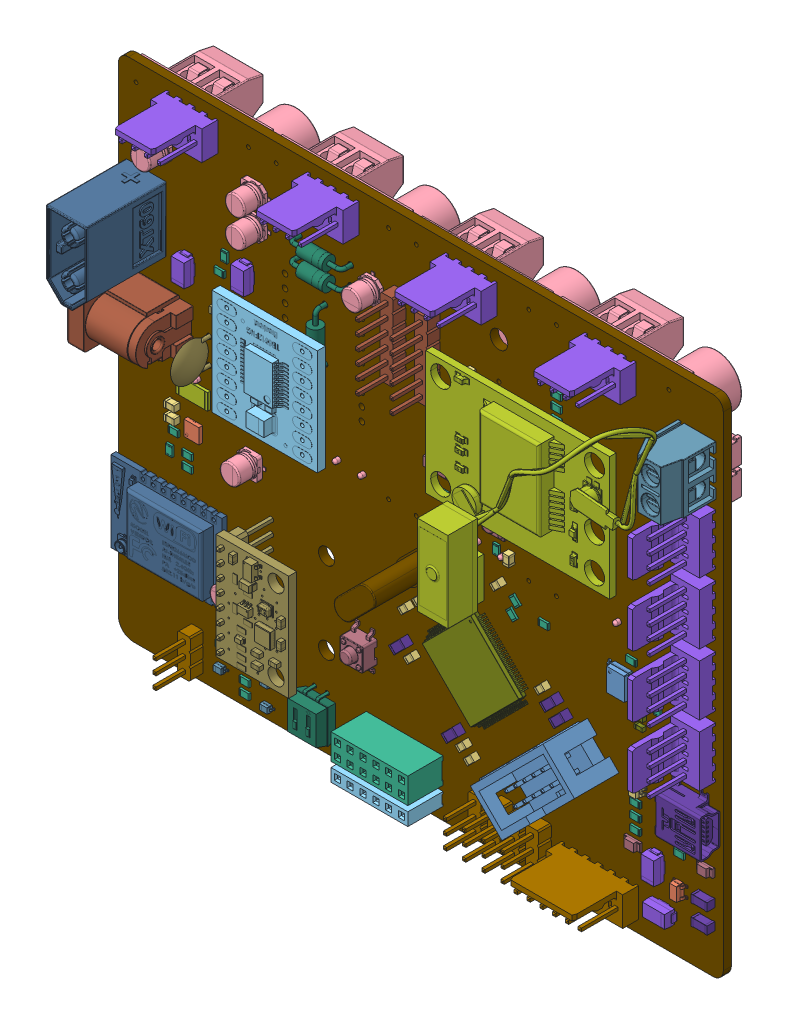
SolidWorks assembly noah_v02, configuration Default. Lengths in mm.
Overall size (125.96 104.91 49.76).
240 component instances, 36 part files, 0 mates.
Components (placement in the parent):
- noah_v02.step-1: noah_v02.step [Default] at origin size (125.96 104.91 49.76)
  - IDC-Header_2x05_P2.54mm_Vertical.step-1: IDC-Header_2x05_P2.54mm_Vertical.step [Default] at (176.6 -132.6 1.65) x (-0.707107 0.707107 0) z (0 0 1) size (9.1 20.36 12.1)
    - SOLID.step-1: SOLID.step [Default] at origin size (9.1 20.36 12.1)
  - DFN-8-1EP_3x3mm_P0.5mm_EP1.66x2.38mm.step-1: DFN-8-1EP_3x3mm_P0.5mm_EP1.66x2.38mm.step [Default] at (105.305 -107.385 1.65) x (0 1 0) z (0 0 1) size (3 2.98 0.77)
    - SOLID-0.step-1: SOLID-0.step [Default] at origin size (3 2.98 0.77)
  - C_0805_2012Metric.step-1: C_0805_2012Metric.step [Default] at (160.4 -70.1 1.65) x (0 -1 0) z (0 0 1) size (2 1.25 1.25)
    - SOLID-1.step-1: SOLID-1.step [Default] at origin size (2 1.25 1.25)
  - CP_Elec_4x4.5.step-1: CP_Elec_4x4.5.step [Default] at (140.6 -65.3 1.65) x (0 -1 0) z (0 0 1) size (5.74 5.46 4.5)
    - SOLID-2.step-1: SOLID-2.step [Default] at origin size (5.74 5.46 4.5)
  - C_0805_2012Metric.step-2: C_0805_2012Metric.step [Default] at (115.6 -134.6 1.65) size (2 1.25 1.25)
    - SOLID-1.step-1: SOLID-1.step [Default] at origin size (2 1.25 1.25)
  - CP_Elec_4x4.5.step-2: CP_Elec_4x4.5.step [Default] at (114.6 -129.4 1.65) x (0 1 0) z (0 0 1) size (5.74 5.46 4.5)
    - SOLID-2.step-1: SOLID-2.step [Default] at origin size (5.74 5.46 4.5)
  - PinSocket_1x06_P2.54mm_Vertical.step-1: PinSocket_1x06_P2.54mm_Vertical.step [Default] at (153.2 -146.2 1.65) x (0 -1 0) z (0 0 1) size (2.54 15.24 10.1)
    - SOLID-3.step-1: SOLID-3.step [Default] at origin size (2.54 15.24 10.1)
  - PinSocket_2x06_P2.54mm_Vertical.step-1: PinSocket_2x06_P2.54mm_Vertical.step [Default] at (153.2 -142.6 1.65) x (0 -1 0) z (0 0 1) size (5.08 15.24 10.1)
    - SOLID-4.step-1: SOLID-4.step [Default] at origin size (5.08 15.24 10.1)
  - ublox_NEO-6M.step-1: ublox_NEO-6M.step [Default] at (181.8 -59.6 11.65) x (0 1 0) z (1 0 0) size (39.06 22.61 48.01)
    - COMPOUND.step-1: COMPOUND.step [Default] at origin size (39.06 22.61 48.01)
  - D_SMA.step-1: D_SMA.step [Default] at (198.4 -143.2 1.65) x (-1 0 0) z (0 0 1) size (5 2.7 2.22)
    - SOLID-5.step-1: SOLID-5.step [Default] at origin size (5 2.7 2.22)
  - PinHeader_1x03_P2.54mm_Vertical.step-1: PinHeader_1x03_P2.54mm_Vertical.step [Default] at (105.6 -147.4 1.65) x (-1 0 0) z (0 0 1) size (2.54 7.62 11.54)
    - SOLID-6.step-1: SOLID-6.step [Default] at origin size (2.54 7.62 11.54)
  - C_0805_2012Metric.step-3: C_0805_2012Metric.step [Default] at (101.3 -107.1 1.65) x (-1 0 0) z (0 0 1) size (2 1.25 1.25)
    - SOLID-1.step-1: SOLID-1.step [Default] at origin size (2 1.25 1.25)
  - C_0805_2012Metric.step-4: C_0805_2012Metric.step [Default] at (101.3 -104.8 1.65) x (-1 0 0) z (0 0 1) size (2 1.25 1.25)
    - SOLID-1.step-1: SOLID-1.step [Default] at origin size (2 1.25 1.25)
  - ESP07.step-1: ESP07.step [Default] at (101.6 -127.3 1.65) x (0 1 0) z (1 0 0) size (19.34 14.61 27.24)
    - COMPOUND-7.step-1: COMPOUND-7.step [Default] at origin size (19.34 14.61 27.24)
  - Power_Barrel_Connector_Jack_694106301002.step-1: Power_Barrel_Connector_Jack_694106301002.step [Default] at (104.13 -90.01 1.65) x (0 -1 0) z (0 0 1) size (9.49 14.48 14.52)
    - COMPOUND-8.step-1: COMPOUND-8.step [Default] at origin size (9.49 14.48 14.52)
  - GY-91.step-1: GY-91.step [Default] at (119 -134.7 9.65) size (14.4 21 11.75)
    - COMPOUND-9.step-1: COMPOUND-9.step [Default] at origin size (14.4 21 11.75)
  - Tact_Switch_4.5mm_SMT.step-1: Tact_Switch_4.5mm_SMT.step [Default] at (139.14 -127.61 1.65) x (0 1 0) z (0 0 1) size (7.5 4.5 4.2)
    - COMPOUND-10.step-1: COMPOUND-10.step [Default] at origin size (7.5 4.5 4.2)
  - Tact_Switch_4.5mm_SMT.step-2: Tact_Switch_4.5mm_SMT.step [Default] at (167.3 -90.93 1.65) x (0 -1 0) z (0 0 1) size (7.5 4.5 4.2)
    - COMPOUND-10.step-1: COMPOUND-10.step [Default] at origin size (7.5 4.5 4.2)
  - tb5p-2p_p5_l10_w7-6_h10.step-1: tb5p-2p_p5_l10_w7-6_h10.step [Default] at (205.55 -62.68 6.65) x (0 1 0) z (1 0 0) size (10.6 14.1 7.6)
    - COMPOUND-11.step-1: COMPOUND-11.step [Default] at origin size (10.6 14.1 7.6)
  - SW_DIP_SPSTx02_Slide_6.7x6.64mm_W7.62mm_P2.54mm_LowProfile.step-1: SW_DIP_SPSTx02_Slide_6.7x6.64mm_W7.62mm_P2.54mm_LowProfile.step [Default] at (131.45 -139.55 1.65) x (-1 0 0) z (0 0 1) size (6.64 7.82 6)
    - SOLID-12.step-1: SOLID-12.step [Default] at origin size (6.64 7.82 6)
  - LQFP-100_14x14mm_P0.5mm.step-1: LQFP-100_14x14mm_P0.5mm.step [Default] at (161.4 -120.1 1.65) x (0.707107 -0.707107 0) z (0 0 1) size (16 16 1.5)
    - SOLID-13.step-1: SOLID-13.step [Default] at origin size (16 16 1.5)
  - USB_Mini-B_Lumberg_2486_01_Horizontal.step-1: USB_Mini-B_Lumberg_2486_01_Horizontal.step [Default] at (203.6 -123.9 1.65) x (0 1 0) z (0 0 1) size (9.9 9.21 5)
    - SOLID-14.step-1: SOLID-14.step [Default] at origin size (9.9 9.21 5)
  - Crystal_HC49-U_Vertical.step-1: Crystal_HC49-U_Vertical.step [Default] at (151.7 -106.6 1.65) x (-0.707107 -0.707107 0) z (0 0 1) size (10.9 4.65 16)
    - SOLID-15.step-1: SOLID-15.step [Default] at origin size (10.9 4.65 16)
  - SOIC-8_3.9x4.9mm_P1.27mm.step-1: SOIC-8_3.9x4.9mm_P1.27mm.step [Default] at (190.4 -107.7 1.65) size (6 4.9 1.75)
    - SOLID-16.step-1: SOLID-16.step [Default] at origin size (6 4.9 1.75)
  - SOT-23-5.step-1: SOT-23-5.step [Default] at (201.6 -138 1.65) size (2.8 2.9 1.55)
    - SOLID-17.step-1: SOLID-17.step [Default] at origin size (2.8 2.9 1.55)
  - SOT-23-6.step-1: SOT-23-6.step [Default] at (193.5 -124.3 1.65) size (2.8 2.9 1.55)
    - SOLID-18.step-1: SOLID-18.step [Default] at origin size (2.8 2.9 1.55)
  - XL4015_StepDown_DC-DC_5A_(CC-CV)_v1.step-1: XL4015_StepDown_DC-DC_5A_(CC-CV)_v1.step [Default] at (119.3 -102.3 -0.05) x (0 1 0) z (0 0 -1) size (51 26 18.15)
    - COMPOUND-19.step-1: COMPOUND-19.step [Default] at origin size (51 26 18.15)
  - XL4015_StepDown_DC-DC_5A_(CC-CV)_v1.step-2: XL4015_StepDown_DC-DC_5A_(CC-CV)_v1.step [Default] at (147.1 -102.4 -0.05) x (0 1 0) z (0 0 -1) size (51 26 18.15)
    - COMPOUND-19.step-1: COMPOUND-19.step [Default] at origin size (51 26 18.15)
  - XL4015_StepDown_DC-DC_5A_(CC-CV)_v1.step-3: XL4015_StepDown_DC-DC_5A_(CC-CV)_v1.step [Default] at (174.9 -102.3 -0.05) x (0 1 0) z (0 0 -1) size (51 26 18.15)
    - COMPOUND-19.step-1: COMPOUND-19.step [Default] at origin size (51 26 18.15)
  - XL4015_StepDown_DC-DC_5A_(CC-CV)_v1.step-4: XL4015_StepDown_DC-DC_5A_(CC-CV)_v1.step [Default] at (91.5 -102.3 -0.05) x (0 1 0) z (0 0 -1) size (51 26 18.15)
    - COMPOUND-19.step-1: COMPOUND-19.step [Default] at origin size (51 26 18.15)
  - TB6612FNG_Motor_Driver.step-1: TB6612FNG_Motor_Driver.step [Default] at (130.68 -80.59 11.65) x (0 0 1) z (1 0 0) size (3.57 20.98 20.9)
    - SOLID-20.step-1: SOLID-20.step [Default] at origin size (3.57 20.98 20.9)
  - R_0805_2012Metric.step-1: R_0805_2012Metric.step [Default] at (168.4 -107.4 1.65) x (0.707107 -0.707107 0) z (0 0 1) size (2 1.2 0.45)
    - SOLID-21.step-1: SOLID-21.step [Default] at origin size (2 1.2 0.45)
  - R_0805_2012Metric.step-2: R_0805_2012Metric.step [Default] at (200.7 -105.4 1.65) x (0 1 0) z (0 0 1) size (2 1.2 0.45)
    - SOLID-21.step-1: SOLID-21.step [Default] at origin size (2 1.2 0.45)
  - R_0805_2012Metric.step-3: R_0805_2012Metric.step [Default] at (200.7 -109.4 1.65) x (0 -1 0) z (0 0 1) size (2 1.2 0.45)
    - SOLID-21.step-1: SOLID-21.step [Default] at origin size (2 1.2 0.45)
  - R_0805_2012Metric.step-4: R_0805_2012Metric.step [Default] at (197.3 -105.4 1.65) x (0 1 0) z (0 0 1) size (2 1.2 0.45)
    - SOLID-21.step-1: SOLID-21.step [Default] at origin size (2 1.2 0.45)
  - R_0805_2012Metric.step-5: R_0805_2012Metric.step [Default] at (197.3 -109.4 1.65) x (0 -1 0) z (0 0 1) size (2 1.2 0.45)
    - SOLID-21.step-1: SOLID-21.step [Default] at origin size (2 1.2 0.45)
  - R_0805_2012Metric.step-6: R_0805_2012Metric.step [Default] at (192.1 -103.5 1.65) size (2 1.2 0.45)
    - SOLID-21.step-1: SOLID-21.step [Default] at origin size (2 1.2 0.45)
  - R_0805_2012Metric.step-7: R_0805_2012Metric.step [Default] at (201.6 -131.9 1.65) x (-1 0 0) z (0 0 1) size (2 1.2 0.45)
    - SOLID-21.step-1: SOLID-21.step [Default] at origin size (2 1.2 0.45)
  - R_0805_2012Metric.step-8: R_0805_2012Metric.step [Default] at (193.5 -120.9 1.65) size (2 1.2 0.45)
    - SOLID-21.step-1: SOLID-21.step [Default] at origin size (2 1.2 0.45)
  - R_0805_2012Metric.step-9: R_0805_2012Metric.step [Default] at (192.9 -127.5 1.65) x (-1 0 0) z (0 0 1) size (2 1.2 0.45)
    - SOLID-21.step-1: SOLID-21.step [Default] at origin size (2 1.2 0.45)
  - R_0805_2012Metric.step-10: R_0805_2012Metric.step [Default] at (192.9 -129.9 1.65) size (2 1.2 0.45)
    - SOLID-21.step-1: SOLID-21.step [Default] at origin size (2 1.2 0.45)
  - R_0805_2012Metric.step-11: R_0805_2012Metric.step [Default] at (110.6 -141.6 1.65) size (2 1.2 0.45)
    - SOLID-21.step-1: SOLID-21.step [Default] at origin size (2 1.2 0.45)
  - R_0805_2012Metric.step-12: R_0805_2012Metric.step [Default] at (177.2 -71.9 1.65) x (-1 0 0) z (0 0 1) size (2 1.2 0.45)
    - SOLID-21.step-1: SOLID-21.step [Default] at origin size (2 1.2 0.45)
  - R_0805_2012Metric.step-13: R_0805_2012Metric.step [Default] at (177.2 -65.3 1.65) x (-1 0 0) z (0 0 1) size (2 1.2 0.45)
    - SOLID-21.step-1: SOLID-21.step [Default] at origin size (2 1.2 0.45)
  - R_0805_2012Metric.step-14: R_0805_2012Metric.step [Default] at (177.2 -69.7 1.65) x (-1 0 0) z (0 0 1) size (2 1.2 0.45)
    - SOLID-21.step-1: SOLID-21.step [Default] at origin size (2 1.2 0.45)
  - R_0805_2012Metric.step-15: R_0805_2012Metric.step [Default] at (177.2 -67.5 1.65) x (-1 0 0) z (0 0 1) size (2 1.2 0.45)
    - SOLID-21.step-1: SOLID-21.step [Default] at origin size (2 1.2 0.45)
  - R_0805_2012Metric.step-16: R_0805_2012Metric.step [Default] at (165.3 -97.8 1.65) x (0 1 0) z (0 0 1) size (2 1.2 0.45)
    - SOLID-21.step-1: SOLID-21.step [Default] at origin size (2 1.2 0.45)
  - R_0805_2012Metric.step-17: R_0805_2012Metric.step [Default] at (152.4 -93.8 1.65) x (0 -1 0) z (0 0 1) size (2 1.2 0.45)
    - SOLID-21.step-1: SOLID-21.step [Default] at origin size (2 1.2 0.45)
  - R_0805_2012Metric.step-18: R_0805_2012Metric.step [Default] at (155.2 -93.8 1.65) x (0 -1 0) z (0 0 1) size (2 1.2 0.45)
    - SOLID-21.step-1: SOLID-21.step [Default] at origin size (2 1.2 0.45)
  - R_0805_2012Metric.step-19: R_0805_2012Metric.step [Default] at (192.9 -132.2 1.65) x (-1 0 0) z (0 0 1) size (2 1.2 0.45)
    - SOLID-21.step-1: SOLID-21.step [Default] at origin size (2 1.2 0.45)
  - R_0805_2012Metric.step-20: R_0805_2012Metric.step [Default] at (169 -104.8 1.65) x (0.707107 -0.707107 0) z (0 0 1) size (2 1.2 0.45)
    - SOLID-21.step-1: SOLID-21.step [Default] at origin size (2 1.2 0.45)
  - R_0805_2012Metric.step-21: R_0805_2012Metric.step [Default] at (174.7 -105.9 1.65) size (2 1.2 0.45)
    - SOLID-21.step-1: SOLID-21.step [Default] at origin size (2 1.2 0.45)
  - R_0805_2012Metric.step-22: R_0805_2012Metric.step [Default] at (111.4 -74.4 1.65) x (0 1 0) z (0 0 1) size (2 1.2 0.45)
    - SOLID-21.step-1: SOLID-21.step [Default] at origin size (2 1.2 0.45)
  - R_0805_2012Metric.step-23: R_0805_2012Metric.step [Default] at (110.4 -77.6 1.65) x (-1 0 0) z (0 0 1) size (2 1.2 0.45)
    - SOLID-21.step-1: SOLID-21.step [Default] at origin size (2 1.2 0.45)
  - R_0805_2012Metric.step-24: R_0805_2012Metric.step [Default] at (101.3 -109.5 1.65) size (2 1.2 0.45)
    - SOLID-21.step-1: SOLID-21.step [Default] at origin size (2 1.2 0.45)
  - R_0805_2012Metric.step-25: R_0805_2012Metric.step [Default] at (100.5 -113.1 1.65) x (0 -1 0) z (0 0 1) size (2 1.2 0.45)
    - SOLID-21.step-1: SOLID-21.step [Default] at origin size (2 1.2 0.45)
  - R_0805_2012Metric.step-26: R_0805_2012Metric.step [Default] at (115.4 -147.6 1.65) size (2 1.2 0.45)
    - SOLID-21.step-1: SOLID-21.step [Default] at origin size (2 1.2 0.45)
  - R_0805_2012Metric.step-27: R_0805_2012Metric.step [Default] at (115.4 -145.4 1.65) size (2 1.2 0.45)
    - SOLID-21.step-1: SOLID-21.step [Default] at origin size (2 1.2 0.45)
  - R_0805_2012Metric.step-28: R_0805_2012Metric.step [Default] at (115.4 -143.2 1.65) size (2 1.2 0.45)
    - SOLID-21.step-1: SOLID-21.step [Default] at origin size (2 1.2 0.45)
  - R_0805_2012Metric.step-29: R_0805_2012Metric.step [Default] at (115.4 -141 1.65) size (2 1.2 0.45)
    - SOLID-21.step-1: SOLID-21.step [Default] at origin size (2 1.2 0.45)
  - R_2512_6332Metric.step-1: R_2512_6332Metric.step [Default] at (105.2 -100.8 1.65) size (6.3 3.2 0.6)
    - SOLID-22.step-1: SOLID-22.step [Default] at origin size (6.3 3.2 0.6)
  - R_0805_2012Metric.step-30: R_0805_2012Metric.step [Default] at (104 -112.2 1.65) x (-1 0 0) z (0 0 1) size (2 1.2 0.45)
    - SOLID-21.step-1: SOLID-21.step [Default] at origin size (2 1.2 0.45)
  - R_0805_2012Metric.step-31: R_0805_2012Metric.step [Default] at (104 -114.4 1.65) x (-1 0 0) z (0 0 1) size (2 1.2 0.45)
    - SOLID-21.step-1: SOLID-21.step [Default] at origin size (2 1.2 0.45)
  - R_0805_2012Metric.step-32: R_0805_2012Metric.step [Default] at (118.1 -81.9 1.65) x (-1 0 0) z (0 0 1) size (2 1.2 0.45)
    - SOLID-21.step-1: SOLID-21.step [Default] at origin size (2 1.2 0.45)
  - Molex_KK-254_AE-6410-04A_1x04_P2.54mm_Vertical.step-1: Molex_KK-254_AE-6410-04A_1x04_P2.54mm_Vertical.step [Default] at (205.6 -95.2 1.65) x (0 -1 0) z (0 0 1) size (10.16 5.8 15.26)
    - SOLID-23.step-1: SOLID-23.step [Default] at origin size (10.16 5.8 15.26)
  - Molex_KK-254_AE-6410-06A_1x06_P2.54mm_Vertical.step-1: Molex_KK-254_AE-6410-06A_1x06_P2.54mm_Vertical.step [Default] at (192 -144.6 1.65) x (-1 0 0) z (0 0 1) size (15.24 5.8 15.26)
    - SOLID-24.step-1: SOLID-24.step [Default] at origin size (15.24 5.8 15.26)
  - Molex_KK-254_AE-6410-04A_1x04_P2.54mm_Vertical.step-2: Molex_KK-254_AE-6410-04A_1x04_P2.54mm_Vertical.step [Default] at (205.6 -70.8 1.65) x (0 -1 0) z (0 0 1) size (10.16 5.8 15.26)
    - SOLID-23.step-1: SOLID-23.step [Default] at origin size (10.16 5.8 15.26)
  - Molex_KK-254_AE-6410-04A_1x04_P2.54mm_Vertical.step-3: Molex_KK-254_AE-6410-04A_1x04_P2.54mm_Vertical.step [Default] at (205.6 -107.4 1.65) x (0 -1 0) z (0 0 1) size (10.16 5.8 15.26)
    - SOLID-23.step-1: SOLID-23.step [Default] at origin size (10.16 5.8 15.26)
  - Molex_KK-254_AE-6410-04A_1x04_P2.54mm_Vertical.step-4: Molex_KK-254_AE-6410-04A_1x04_P2.54mm_Vertical.step [Default] at (205.6 -83 1.65) x (0 -1 0) z (0 0 1) size (10.16 5.8 15.26)
    - SOLID-23.step-1: SOLID-23.step [Default] at origin size (10.16 5.8 15.26)
  - PinHeader_1x03_P2.54mm_Vertical.step-2: PinHeader_1x03_P2.54mm_Vertical.step [Default] at (163.25 -146.15 1.65) x (-1 0 0) z (0 0 1) size (2.54 7.62 11.54)
    - SOLID-6.step-1: SOLID-6.step [Default] at origin size (2.54 7.62 11.54)
  - PinHeader_1x03_P2.54mm_Vertical.step-3: PinHeader_1x03_P2.54mm_Vertical.step [Default] at (167.05 -146.15 1.65) x (-1 0 0) z (0 0 1) size (2.54 7.62 11.54)
    - SOLID-6.step-1: SOLID-6.step [Default] at origin size (2.54 7.62 11.54)
  - PinHeader_1x03_P2.54mm_Vertical.step-4: PinHeader_1x03_P2.54mm_Vertical.step [Default] at (170.85 -146.15 1.65) x (-1 0 0) z (0 0 1) size (2.54 7.62 11.54)
    - SOLID-6.step-1: SOLID-6.step [Default] at origin size (2.54 7.62 11.54)
  - PinHeader_1x03_P2.54mm_Vertical.step-5: PinHeader_1x03_P2.54mm_Vertical.step [Default] at (174.65 -146.15 1.65) x (-1 0 0) z (0 0 1) size (2.54 7.62 11.54)
    - SOLID-6.step-1: SOLID-6.step [Default] at origin size (2.54 7.62 11.54)
  - Molex_KK-254_AE-6410-04A_1x04_P2.54mm_Vertical.step-5: Molex_KK-254_AE-6410-04A_1x04_P2.54mm_Vertical.step [Default] at (108.5 -54.8 1.65) x (-1 0 0) z (0 0 1) size (10.16 5.8 15.26)
    - SOLID-23.step-1: SOLID-23.step [Default] at origin size (10.16 5.8 15.26)
  - Molex_KK-254_AE-6410-04A_1x04_P2.54mm_Vertical.step-6: Molex_KK-254_AE-6410-04A_1x04_P2.54mm_Vertical.step [Default] at (163.9 -55 1.65) x (-1 0 0) z (0 0 1) size (10.16 5.8 15.26)
    - SOLID-23.step-1: SOLID-23.step [Default] at origin size (10.16 5.8 15.26)
  - XT60_Male_Connector.step-1: XT60_Male_Connector.step [Default] at (95.7 -75.4 17.65) x (0 1 0) z (-1 0 0) size (15.93 20.03 8.13)
    - COMPOUND-25.step-1: COMPOUND-25.step [Default] at origin size (15.93 20.03 8.13)
  - Molex_KK-254_AE-6410-04A_1x04_P2.54mm_Vertical.step-7: Molex_KK-254_AE-6410-04A_1x04_P2.54mm_Vertical.step [Default] at (136.5 -54.8 1.65) x (-1 0 0) z (0 0 1) size (10.16 5.8 15.26)
    - SOLID-23.step-1: SOLID-23.step [Default] at origin size (10.16 5.8 15.26)
  - Molex_KK-254_AE-6410-04A_1x04_P2.54mm_Vertical.step-8: Molex_KK-254_AE-6410-04A_1x04_P2.54mm_Vertical.step [Default] at (191.5 -54.9 1.65) x (-1 0 0) z (0 0 1) size (10.16 5.8 15.26)
    - SOLID-23.step-1: SOLID-23.step [Default] at origin size (10.16 5.8 15.26)
  - PinHeader_1x06_P2.54mm_Vertical.step-1: PinHeader_1x06_P2.54mm_Vertical.step [Default] at (152.6 -76.7 1.65) x (-1 0 0) z (0 0 1) size (2.54 15.24 11.54)
    - SOLID-26.step-1: SOLID-26.step [Default] at origin size (2.54 15.24 11.54)
  - PinHeader_1x06_P2.54mm_Vertical.step-2: PinHeader_1x06_P2.54mm_Vertical.step [Default] at (145.8 -76.74 1.65) x (-1 0 0) z (0 0 1) size (2.54 15.24 11.54)
    - SOLID-26.step-1: SOLID-26.step [Default] at origin size (2.54 15.24 11.54)
  - C_Disc_D7.5mm_W2.5mm_P5.00mm.step-1: C_Disc_D7.5mm_W2.5mm_P5.00mm.step [Default] at (108 -95 1.65) x (0 1 0) z (0 0 1) size (7.5 2.5 9.6)
    - SOLID-27.step-1: SOLID-27.step [Default] at origin size (7.5 2.5 9.6)
  - LED_1206_3216Metric.step-1: LED_1206_3216Metric.step [Default] at (206.8 -131.9 1.65) x (-1 0 0) z (0 0 1) size (3.2 1.6 1.1)
    - SOLID-28.step-1: SOLID-28.step [Default] at origin size (3.2 1.6 1.1)
  - D_SMA.step-2: D_SMA.step [Default] at (197.2 -136 1.65) x (0 1 0) z (0 0 1) size (5 2.7 2.22)
    - SOLID-5.step-1: SOLID-5.step [Default] at origin size (5 2.7 2.22)
  - D_SOD-323.step-1: D_SOD-323.step [Default] at (119.9 -147.5 1.65) size (2.5 1.25 1.1)
    - SOLID-29.step-1: SOLID-29.step [Default] at origin size (2.5 1.25 1.1)
  - D_SMA.step-3: D_SMA.step [Default] at (113.8 -95 1.65) x (-1 0 0) z (0 0 1) size (5 2.7 2.22)
    - SOLID-5.step-1: SOLID-5.step [Default] at origin size (5 2.7 2.22)
  - D_SMA.step-4: D_SMA.step [Default] at (115.8 -75.4 1.65) x (0 1 0) z (0 0 1) size (5 2.7 2.22)
    - SOLID-5.step-1: SOLID-5.step [Default] at origin size (5 2.7 2.22)
  - D_SMA.step-5: D_SMA.step [Default] at (104 -79.9 1.65) x (0 1 0) z (0 0 1) size (5 2.7 2.22)
    - SOLID-5.step-1: SOLID-5.step [Default] at origin size (5 2.7 2.22)
  - LED_1206_3216Metric.step-2: LED_1206_3216Metric.step [Default] at (152.4 -89 1.65) x (0 -1 0) z (0 0 1) size (3.2 1.6 1.1)
    - SOLID-28.step-1: SOLID-28.step [Default] at origin size (3.2 1.6 1.1)
  - LED_1206_3216Metric.step-3: LED_1206_3216Metric.step [Default] at (155.2 -89 1.65) x (0 -1 0) z (0 0 1) size (3.2 1.6 1.1)
    - SOLID-28.step-1: SOLID-28.step [Default] at origin size (3.2 1.6 1.1)
  - LED_1206_3216Metric.step-4: LED_1206_3216Metric.step [Default] at (192.4 -134.7 1.65) size (3.2 1.6 1.1)
    - SOLID-28.step-1: SOLID-28.step [Default] at origin size (3.2 1.6 1.1)
  - D_SOD-323.step-2: D_SOD-323.step [Default] at (110.7 -145.4 1.65) size (2.5 1.25 1.1)
    - SOLID-29.step-1: SOLID-29.step [Default] at origin size (2.5 1.25 1.1)
  - D_SOD-323.step-3: D_SOD-323.step [Default] at (119.9 -143.2 1.65) size (2.5 1.25 1.1)
    - SOLID-29.step-1: SOLID-29.step [Default] at origin size (2.5 1.25 1.1)
  - D_DO-41_SOD81_P10.16mm_Horizontal.step-1: D_DO-41_SOD81_P10.16mm_Horizontal.step [Default] at (131 -83.2 1.65) x (0 1 0) z (0 0 1) size (10.96 2.72 5.71)
    - SOLID-30.step-1: SOLID-30.step [Default] at origin size (10.96 2.72 5.71)
  - D_DO-41_SOD81_P10.16mm_Horizontal.step-2: D_DO-41_SOD81_P10.16mm_Horizontal.step [Default] at (136.1 -67.3 1.65) x (-1 0 0) z (0 0 1) size (10.96 2.72 5.71)
    - SOLID-30.step-1: SOLID-30.step [Default] at origin size (10.96 2.72 5.71)
  - D_DO-41_SOD81_P10.16mm_Horizontal.step-3: D_DO-41_SOD81_P10.16mm_Horizontal.step [Default] at (136.1 -63.7 1.65) x (-1 0 0) z (0 0 1) size (10.96 2.72 5.71)
    - SOLID-30.step-1: SOLID-30.step [Default] at origin size (10.96 2.72 5.71)
  - C_0805_2012Metric.step-5: C_0805_2012Metric.step [Default] at (160.8 -135.8 1.65) x (-0.707107 -0.707107 0) z (0 0 1) size (2 1.25 1.25)
    - SOLID-1.step-1: SOLID-1.step [Default] at origin size (2 1.25 1.25)
  - C_0603_1608Metric.step-1: C_0603_1608Metric.step [Default] at (193.96 -113.92 1.65) x (-1 0 0) z (0 0 1) size (1.6 0.8 0.8)
    - SOLID-31.step-1: SOLID-31.step [Default] at origin size (1.6 0.8 0.8)
  - C_0603_1608Metric.step-2: C_0603_1608Metric.step [Default] at (194 -112.2 1.65) x (-1 0 0) z (0 0 1) size (1.6 0.8 0.8)
    - SOLID-31.step-1: SOLID-31.step [Default] at origin size (1.6 0.8 0.8)
  - C_1206_3216Metric.step-1: C_1206_3216Metric.step [Default] at (206.8 -137.1 1.65) size (3.2 1.6 1.6)
    - SOLID-32.step-1: SOLID-32.step [Default] at origin size (3.2 1.6 1.6)
  - C_1206_3216Metric.step-2: C_1206_3216Metric.step [Default] at (206.8 -141.1 1.65) size (3.2 1.6 1.6)
    - SOLID-32.step-1: SOLID-32.step [Default] at origin size (3.2 1.6 1.6)
  - CP_Elec_4x4.5.step-3: CP_Elec_4x4.5.step [Default] at (116.6 -107.2 1.65) size (5.74 5.46 4.5)
    - SOLID-2.step-1: SOLID-2.step [Default] at origin size (5.74 5.46 4.5)
  - CP_Elec_4x4.5.step-4: CP_Elec_4x4.5.step [Default] at (98.8 -62 1.65) x (-1 0 0) z (0 0 1) size (5.74 5.46 4.5)
    - SOLID-2.step-1: SOLID-2.step [Default] at origin size (5.74 5.46 4.5)
  - C_0805_2012Metric.step-6: C_0805_2012Metric.step [Default] at (110.3 -84.1 1.65) size (2 1.25 1.25)
    - SOLID-1.step-1: SOLID-1.step [Default] at origin size (2 1.25 1.25)
  - CP_Elec_4x4.5.step-5: CP_Elec_4x4.5.step [Default] at (117.6 -60.5 1.65) x (-1 0 0) z (0 0 1) size (5.74 5.46 4.5)
    - SOLID-2.step-1: SOLID-2.step [Default] at origin size (5.74 5.46 4.5)
  - C_0805_2012Metric.step-7: C_0805_2012Metric.step [Default] at (168.1 -97.8 1.65) x (0 1 0) z (0 0 1) size (2 1.25 1.25)
    - SOLID-1.step-1: SOLID-1.step [Default] at origin size (2 1.25 1.25)
  - C_1206_3216Metric.step-3: C_1206_3216Metric.step [Default] at (176.8 -118 1.65) x (0.707107 0.707107 0) z (0 0 1) size (3.2 1.6 1.6)
    - SOLID-32.step-1: SOLID-32.step [Default] at origin size (3.2 1.6 1.6)
  - C_1206_3216Metric.step-4: C_1206_3216Metric.step [Default] at (178.6 -119.9 1.65) x (0.707107 0.707107 0) z (0 0 1) size (3.2 1.6 1.6)
    - SOLID-32.step-1: SOLID-32.step [Default] at origin size (3.2 1.6 1.6)
  - C_1206_3216Metric.step-5: C_1206_3216Metric.step [Default] at (157.3 -133.1 1.65) x (-0.707107 -0.707107 0) z (0 0 1) size (3.2 1.6 1.6)
    - SOLID-32.step-1: SOLID-32.step [Default] at origin size (3.2 1.6 1.6)
  - C_0603_1608Metric.step-3: C_0603_1608Metric.step [Default] at (145.2 -114.4 1.65) x (0.707107 -0.707107 0) z (0 0 1) size (1.6 0.8 0.8)
    - SOLID-31.step-1: SOLID-31.step [Default] at origin size (1.6 0.8 0.8)
  - C_0603_1608Metric.step-4: C_0603_1608Metric.step [Default] at (156.1 -103.5 1.65) x (0.707107 -0.707107 0) z (0 0 1) size (1.6 0.8 0.8)
    - SOLID-31.step-1: SOLID-31.step [Default] at origin size (1.6 0.8 0.8)
  - C_0805_2012Metric.step-8: C_0805_2012Metric.step [Default] at (150.6 -113.5 1.65) x (-0.707107 -0.707107 0) z (0 0 1) size (2 1.25 1.25)
    - SOLID-1.step-1: SOLID-1.step [Default] at origin size (2 1.25 1.25)
  - C_0805_2012Metric.step-9: C_0805_2012Metric.step [Default] at (147.7 -116.4 1.65) x (0.707107 0.707107 0) z (0 0 1) size (2 1.25 1.25)
    - SOLID-1.step-1: SOLID-1.step [Default] at origin size (2 1.25 1.25)
  - C_0805_2012Metric.step-10: C_0805_2012Metric.step [Default] at (156.6 -108.9 1.65) x (-0.707107 -0.707107 0) z (0 0 1) size (2 1.25 1.25)
    - SOLID-1.step-1: SOLID-1.step [Default] at origin size (2 1.25 1.25)
  - C_1206_3216Metric.step-6: C_1206_3216Metric.step [Default] at (146.9 -123.1 1.65) x (-0.707107 -0.707107 0) z (0 0 1) size (3.2 1.6 1.6)
    - SOLID-32.step-1: SOLID-32.step [Default] at origin size (3.2 1.6 1.6)
  - C_0805_2012Metric.step-11: C_0805_2012Metric.step [Default] at (166 -103.2 1.65) x (0.707107 0.707107 0) z (0 0 1) size (2 1.25 1.25)
    - SOLID-1.step-1: SOLID-1.step [Default] at origin size (2 1.25 1.25)
  - C_0805_2012Metric.step-12: C_0805_2012Metric.step [Default] at (148.9 -124.3 1.65) x (0.707107 0.707107 0) z (0 0 1) size (2 1.25 1.25)
    - SOLID-1.step-1: SOLID-1.step [Default] at origin size (2 1.25 1.25)
  - C_0805_2012Metric.step-13: C_0805_2012Metric.step [Default] at (159.2 -134.3 1.65) x (0.707107 0.707107 0) z (0 0 1) size (2 1.25 1.25)
    - SOLID-1.step-1: SOLID-1.step [Default] at origin size (2 1.25 1.25)
  - C_0805_2012Metric.step-14: C_0805_2012Metric.step [Default] at (174.8 -116.6 1.65) x (-0.707107 -0.707107 0) z (0 0 1) size (2 1.25 1.25)
    - SOLID-1.step-1: SOLID-1.step [Default] at origin size (2 1.25 1.25)
  - CP_Elec_4x4.5.step-6: CP_Elec_4x4.5.step [Default] at (117.6 -66.1 1.65) x (-1 0 0) z (0 0 1) size (5.74 5.46 4.5)
    - SOLID-2.step-1: SOLID-2.step [Default] at origin size (5.74 5.46 4.5)
  - COMPOUND-33.step-1: COMPOUND-33.step [Default] at origin size (120 100 1.6)
